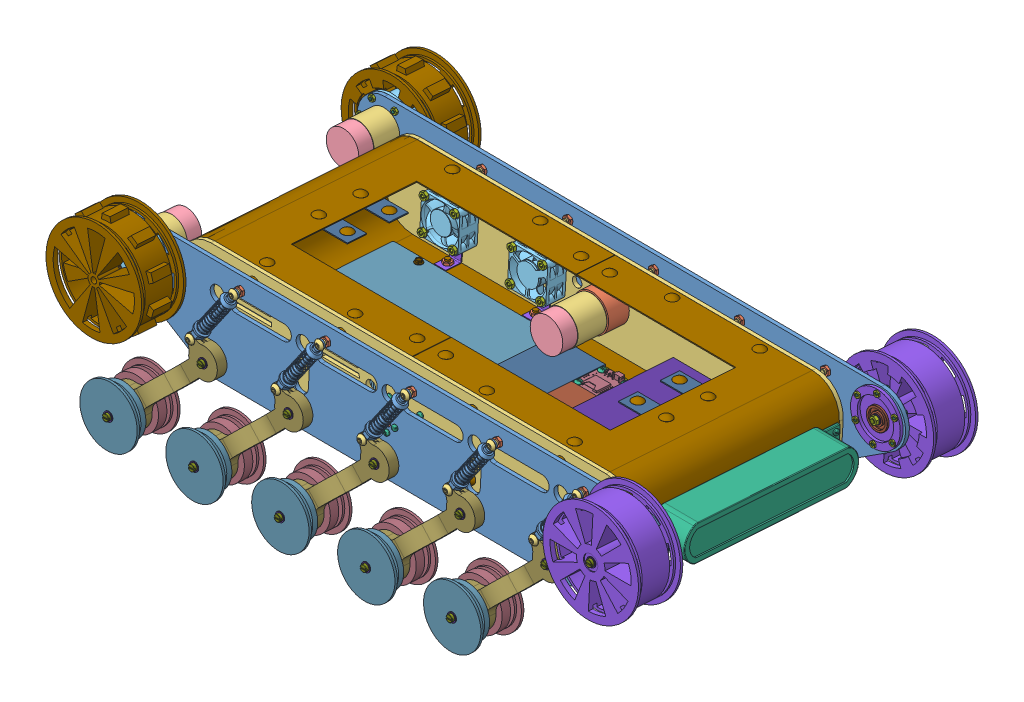
SolidWorks assembly Ensamble_Detallado_2, configuration Predeterminado. Lengths in mm. (continued)
Components (placement in the parent): (continued)
- hex nut jam_am-69: hex nut jam_am [B18.2.4.5M - Hex jam nut,  M5 x 0.8 --D-N] at (182.3196 36.3655 -544.0322) x (0.998179 0.060274 0.002247) z (-0.005872 0.060029 0.998179) size (8 9.24 2.7)
- hex nut jam_am-70: hex nut jam_am [B18.2.4.5M - Hex jam nut,  M5 x 0.8 --D-N] at (92.3211 36.384 -544.5628) x (0.998179 0.060274 0.002247) z (-0.005872 0.060029 0.998179) size (8 9.24 2.7)
- hex nut jam_am-71: hex nut jam_am [B18.2.4.5M - Hex jam nut,  M5 x 0.8 --D-N] at (2.3227 36.4024 -545.0933) x (0.998179 0.060274 0.002247) z (-0.005872 0.060029 0.998179) size (8 9.24 2.7)
- hex nut jam_am-72: hex nut jam_am [B18.2.4.5M - Hex jam nut,  M5 x 0.8 --D-N] at (-87.6757 36.4208 -545.6238) x (0.998179 0.060274 0.002247) z (-0.005872 0.060029 0.998179) size (8 9.24 2.7)
- hex nut jam_am-73: hex nut jam_am [B18.2.4.5M - Hex jam nut,  M5 x 0.8 --D-N] at (182.2802 36.7677 -537.3444) x (0.998179 0.060274 0.002247) z (-0.005872 0.060029 0.998179) size (8 9.24 2.7)
- hex nut jam_am-74: hex nut jam_am [B18.2.4.5M - Hex jam nut,  M5 x 0.8 --D-N] at (92.2818 36.7862 -537.875) x (0.998179 0.060274 0.002247) z (-0.005872 0.060029 0.998179) size (8 9.24 2.7)
- hex nut jam_am-75: hex nut jam_am [B18.2.4.5M - Hex jam nut,  M5 x 0.8 --D-N] at (2.2834 36.8046 -538.4055) x (0.998179 0.060274 0.002247) z (-0.005872 0.060029 0.998179) size (8 9.24 2.7)
- hex nut jam_am-76: hex nut jam_am [B18.2.4.5M - Hex jam nut,  M5 x 0.8 --D-N] at (-87.7151 36.823 -538.936) x (0.998179 0.060274 0.002247) z (-0.005872 0.060029 0.998179) size (8 9.24 2.7)
- Pasador-4: Pasador [Predeterminado] at (98.9679 -93.8939 -530.1771) x (0.998179 0.060274 0.002247) z (-0.005872 0.060029 0.998179) size (8 8 44.5)
- Pasador-5: Pasador [Predeterminado] at (8.9695 -93.8755 -530.7076) x (0.998179 0.060274 0.002247) z (-0.005872 0.060029 0.998179) size (8 8 44.5)
- Pasador-6: Pasador [Predeterminado] at (-81.0289 -93.8571 -531.2382) x (0.998179 0.060274 0.002247) z (-0.005872 0.060029 0.998179) size (8 8 44.5)
- Pasador-7: Pasador [Predeterminado] at (-171.0274 -93.8386 -531.7687) x (0.998179 0.060274 0.002247) z (-0.005872 0.060029 0.998179) size (8 8 44.5)
- Tubo_Pata-2: Tubo_Pata [Predeterminado] at (158.4464 -33.6132 -539.9643) x (0.999983 0.000176 0.005872) z (-0.005872 0.060029 0.998179) size (8 8 11)
- Tubo_Pata-3: Tubo_Pata [Predeterminado] at (68.448 -33.5947 -540.4948) x (0.999983 0.000176 0.005872) z (-0.005872 0.060029 0.998179) size (8 8 11)
- Tubo_Pata-4: Tubo_Pata [Predeterminado] at (-21.5505 -33.5763 -541.0253) x (0.999983 0.000176 0.005872) z (-0.005872 0.060029 0.998179) size (8 8 11)
- Tubo_Pata-5: Tubo_Pata [Predeterminado] at (-111.5489 -33.5579 -541.5558) x (0.999983 0.000176 0.005872) z (-0.005872 0.060029 0.998179) size (8 8 11)
- plain washer - normal_as-30: plain washer - normal_as [AS 1237.1 N - 4] at (100.4952 -109.5074 -789.8036) x (-0.99997 -0.005414 -0.005557) z (0.005872 -0.060029 -0.998179) size (9 9 0.8)
- plain washer - normal_as-31: plain washer - normal_as [AS 1237.1 N - 4] at (10.4967 -109.489 -790.3341) x (-0.99997 -0.005414 -0.005557) z (0.005872 -0.060029 -0.998179) size (9 9 0.8)
- plain washer - normal_as-32: plain washer - normal_as [AS 1237.1 N - 4] at (-79.5017 -109.4705 -790.8646) x (-0.99997 -0.005414 -0.005557) z (0.005872 -0.060029 -0.998179) size (9 9 0.8)
- plain washer - normal_as-33: plain washer - normal_as [AS 1237.1 N - 4] at (-169.5001 -109.4521 -791.3951) x (-0.99997 -0.005414 -0.005557) z (0.005872 -0.060029 -0.998179) size (9 9 0.8)
- Rueda_Resorte2V1.3-20: Rueda_Resorte2V1.3 [Predeterminado] at (100.6067 -110.648 -808.769) x (0.047484 -0.997054 0.06024) z (-0.005872 0.060029 0.998179) size (60 60 20.5)
- Rueda_Resorte2V1.3-21: Rueda_Resorte2V1.3 [Predeterminado] at (10.6083 -110.6295 -809.2995) x (0.047484 -0.997054 0.06024) z (-0.005872 0.060029 0.998179) size (60 60 20.5)
- Rueda_Resorte2V1.3-22: Rueda_Resorte2V1.3 [Predeterminado] at (-79.3901 -110.6111 -809.83) x (0.047484 -0.997054 0.06024) z (-0.005872 0.060029 0.998179) size (60 60 20.5)
- Rueda_Resorte2V1.3-23: Rueda_Resorte2V1.3 [Predeterminado] at (-169.3886 -110.5927 -810.3605) x (0.047484 -0.997054 0.06024) z (-0.005872 0.060029 0.998179) size (60 60 20.5)
- hex nut style 1_am-111: hex nut style 1_am [B18.2.4.1M - Hex nut, Style 1,  M4 x 0.7 --D-N] at (100.4905 -109.4594 -789.005) x (-0.99997 -0.005414 -0.005557) z (0.005872 -0.060029 -0.998179) size (7 8.08 3.2)
- hex nut style 1_am-112: hex nut style 1_am [B18.2.4.1M - Hex nut, Style 1,  M4 x 0.7 --D-N] at (10.492 -109.441 -789.5356) x (-0.99997 -0.005414 -0.005557) z (0.005872 -0.060029 -0.998179) size (7 8.08 3.2)
- hex nut style 1_am-113: hex nut style 1_am [B18.2.4.1M - Hex nut, Style 1,  M4 x 0.7 --D-N] at (-79.5064 -109.4225 -790.0661) x (-0.99997 -0.005414 -0.005557) z (0.005872 -0.060029 -0.998179) size (7 8.08 3.2)
- hex nut style 1_am-114: hex nut style 1_am [B18.2.4.1M - Hex nut, Style 1,  M4 x 0.7 --D-N] at (-169.5048 -109.4041 -790.5966) x (-0.99997 -0.005414 -0.005557) z (0.005872 -0.060029 -0.998179) size (7 8.08 3.2)
- plain washer - normal_as-34: plain washer - normal_as [AS 1237.1 N - 4] at (100.7611 -112.2267 -835.0211) x (-0.99997 -0.005414 -0.005557) z (0.005872 -0.060029 -0.998179) size (9 9 0.8)
- plain washer - normal_as-35: plain washer - normal_as [AS 1237.1 N - 4] at (10.7627 -112.2083 -835.5516) x (-0.99997 -0.005414 -0.005557) z (0.005872 -0.060029 -0.998179) size (9 9 0.8)
- plain washer - normal_as-36: plain washer - normal_as [AS 1237.1 N - 4] at (-79.2357 -112.1898 -836.0821) x (-0.99997 -0.005414 -0.005557) z (0.005872 -0.060029 -0.998179) size (9 9 0.8)
- plain washer - normal_as-37: plain washer - normal_as [AS 1237.1 N - 4] at (-169.2342 -112.1714 -836.6127) x (-0.99997 -0.005414 -0.005557) z (0.005872 -0.060029 -0.998179) size (9 9 0.8)
- cheese head screw_as-16: cheese head screw_as [AS-NZS 1427 CH - M4 x 50-N] at (100.7764 -112.3828 -837.6164) x (-0.005872 0.060029 0.998179) z (-0.99997 -0.005414 -0.005557) size (52.62 7 7)
- cheese head screw_as-17: cheese head screw_as [AS-NZS 1427 CH - M4 x 50-N] at (10.778 -112.3644 -838.1469) x (-0.005872 0.060029 0.998179) z (-0.99997 -0.005414 -0.005557) size (52.62 7 7)
- cheese head screw_as-18: cheese head screw_as [AS-NZS 1427 CH - M4 x 50-N] at (-79.2205 -112.3459 -838.6774) x (-0.005872 0.060029 0.998179) z (-0.99997 -0.005414 -0.005557) size (52.62 7 7)
- cheese head screw_as-19: cheese head screw_as [AS-NZS 1427 CH - M4 x 50-N] at (-169.2189 -112.3275 -839.2079) x (-0.005872 0.060029 0.998179) z (-0.99997 -0.005414 -0.005557) size (52.62 7 7)
- Rueda_ResorteV1.3-24: Rueda_ResorteV1.3 [Predeterminado] at (100.6654 -111.2482 -818.7508) x (0.99997 -0.004709 0.006165) z (0.005872 -0.060029 -0.998179) size (60 60 17)
- Rueda_ResorteV1.3-25: Rueda_ResorteV1.3 [Predeterminado] at (10.667 -111.2298 -819.2813) x (0.99997 -0.004709 0.006165) z (0.005872 -0.060029 -0.998179) size (60 60 17)
- Rueda_ResorteV1.3-26: Rueda_ResorteV1.3 [Predeterminado] at (-79.3314 -111.2114 -819.8118) x (0.99997 -0.004709 0.006165) z (0.005872 -0.060029 -0.998179) size (60 60 17)
- Rueda_ResorteV1.3-27: Rueda_ResorteV1.3 [Predeterminado] at (-169.3299 -111.1929 -820.3423) x (0.99997 -0.004709 0.006165) z (0.005872 -0.060029 -0.998179) size (60 60 17)
- plain washer - normal_as-38: plain washer - normal_as [AS 1237.1 N - 4] at (159.8973 -48.4463 -786.6144) x (-0.998179 -0.060274 -0.002247) z (0.005872 -0.060029 -0.998179) size (9 9 0.8)
- plain washer - normal_as-39: plain washer - normal_as [AS 1237.1 N - 4] at (69.8989 -48.4278 -787.1449) x (-0.998179 -0.060274 -0.002247) z (0.005872 -0.060029 -0.998179) size (9 9 0.8)
- plain washer - normal_as-40: plain washer - normal_as [AS 1237.1 N - 4] at (-20.0996 -48.4094 -787.6754) x (-0.998179 -0.060274 -0.002247) z (0.005872 -0.060029 -0.998179) size (9 9 0.8)
- plain washer - normal_as-41: plain washer - normal_as [AS 1237.1 N - 4] at (-110.098 -48.391 -788.206) x (-0.998179 -0.060274 -0.002247) z (0.005872 -0.060029 -0.998179) size (9 9 0.8)
- hex nut style 1_am-115: hex nut style 1_am [B18.2.4.1M - Hex nut, Style 1,  M4 x 0.7 --D-N] at (159.8926 -48.3982 -785.8159) x (-0.99853 -0.054135 -0.002618) z (0.005872 -0.060029 -0.998179) size (7 8.08 3.2)
- hex nut style 1_am-116: hex nut style 1_am [B18.2.4.1M - Hex nut, Style 1,  M4 x 0.7 --D-N] at (69.8942 -48.3798 -786.3464) x (-0.99853 -0.054135 -0.002618) z (0.005872 -0.060029 -0.998179) size (7 8.08 3.2)
- hex nut style 1_am-117: hex nut style 1_am [B18.2.4.1M - Hex nut, Style 1,  M4 x 0.7 --D-N] at (-20.1043 -48.3614 -786.8769) x (-0.99853 -0.054135 -0.002618) z (0.005872 -0.060029 -0.998179) size (7 8.08 3.2)
- hex nut style 1_am-118: hex nut style 1_am [B18.2.4.1M - Hex nut, Style 1,  M4 x 0.7 --D-N] at (-110.1027 -48.3429 -787.4074) x (-0.99853 -0.054135 -0.002618) z (0.005872 -0.060029 -0.998179) size (7 8.08 3.2)
- plain washer - normal_as-42: plain washer - normal_as [AS 1237.1 N - 4] at (159.993 -49.4247 -802.8847) x (0.958426 -0.284435 0.022743) z (0.005872 -0.060029 -0.998179) size (9 9 0.8)
- plain washer - normal_as-43: plain washer - normal_as [AS 1237.1 N - 4] at (69.9946 -49.4063 -803.4152) x (0.958426 -0.284435 0.022743) z (0.005872 -0.060029 -0.998179) size (9 9 0.8)
- plain washer - normal_as-44: plain washer - normal_as [AS 1237.1 N - 4] at (-20.0039 -49.3879 -803.9458) x (0.958426 -0.284435 0.022743) z (0.005872 -0.060029 -0.998179) size (9 9 0.8)
- plain washer - normal_as-45: plain washer - normal_as [AS 1237.1 N - 4] at (-110.0023 -49.3694 -804.4763) x (0.958426 -0.284435 0.022743) z (0.005872 -0.060029 -0.998179) size (9 9 0.8)
- socket button head cap screw_am-16: socket button head cap screw_am [B18.3.4M - 5 x 0.8 x 10 SBHCS --N] at (145.7758 -35.5561 -805.756) x (-0.005872 0.060029 0.998179) z (-0.100585 -0.993169 0.059136) size (12.75 9.5 9.5)
- socket button head cap screw_am-17: socket button head cap screw_am [B18.3.4M - 5 x 0.8 x 10 SBHCS --N] at (55.7774 -35.5376 -806.2865) x (-0.005872 0.060029 0.998179) z (-0.100585 -0.993169 0.059136) size (12.75 9.5 9.5)
- socket button head cap screw_am-18: socket button head cap screw_am [B18.3.4M - 5 x 0.8 x 10 SBHCS --N] at (-34.2211 -35.5192 -806.817) x (-0.005872 0.060029 0.998179) z (-0.100585 -0.993169 0.059136) size (12.75 9.5 9.5)
- socket button head cap screw_am-19: socket button head cap screw_am [B18.3.4M - 5 x 0.8 x 10 SBHCS --N] at (-124.2195 -35.5008 -807.3475) x (-0.005872 0.060029 0.998179) z (-0.100585 -0.993169 0.059136) size (12.75 9.5 9.5)
- cheese head screw_as-20: cheese head screw_as [AS-NZS 1427 CH - M4 x 20-N] at (160.0083 -49.5808 -805.48) x (-0.005872 0.060029 0.998179) z (0.11687 0.991397 -0.058933) size (22.6 7 7)
- cheese head screw_as-21: cheese head screw_as [AS-NZS 1427 CH - M4 x 20-N] at (70.0098 -49.5624 -806.0105) x (-0.005872 0.060029 0.998179) z (0.11687 0.991397 -0.058933) size (22.6 7 7)
- cheese head screw_as-22: cheese head screw_as [AS-NZS 1427 CH - M4 x 20-N] at (-19.9886 -49.5439 -806.541) x (-0.005872 0.060029 0.998179) z (0.11687 0.991397 -0.058933) size (22.6 7 7)
- cheese head screw_as-23: cheese head screw_as [AS-NZS 1427 CH - M4 x 20-N] at (-109.987 -49.5255 -807.0715) x (-0.005872 0.060029 0.998179) z (0.11687 0.991397 -0.058933) size (22.6 7 7)
- Pieza_Resorte_2V1.5-2: Pieza_Resorte_2V1.5 [Predeterminado] at (100.6361 -110.9481 -813.7599) x (0.005872 -0.060029 -0.998179) z (-0.699298 -0.713776 0.038812) size (30 44.97 120)
- Pieza_Resorte_2V1.5-3: Pieza_Resorte_2V1.5 [Predeterminado] at (10.6376 -110.9297 -814.2904) x (0.005872 -0.060029 -0.998179) z (-0.699298 -0.713776 0.038812) size (30 44.97 120)
- Pieza_Resorte_2V1.5-4: Pieza_Resorte_2V1.5 [Predeterminado] at (-79.3608 -110.9112 -814.8209) x (0.005872 -0.060029 -0.998179) z (-0.699298 -0.713776 0.038812) size (30 44.97 120)
- Pieza_Resorte_2V1.5-5: Pieza_Resorte_2V1.5 [Predeterminado] at (-169.3592 -110.8928 -815.3514) x (0.005872 -0.060029 -0.998179) z (-0.699298 -0.713776 0.038812) size (30 44.97 120)
- hex nut jam_am-77: hex nut jam_am [B18.2.4.5M - Hex jam nut,  M5 x 0.8 --D-N] at (183.7546 21.6945 -787.9873) x (0.998179 0.060274 0.002247) z (-0.005872 0.060029 0.998179) size (8 9.24 2.7)
- hex nut jam_am-78: hex nut jam_am [B18.2.4.5M - Hex jam nut,  M5 x 0.8 --D-N] at (93.7562 21.7129 -788.5178) x (0.998179 0.060274 0.002247) z (-0.005872 0.060029 0.998179) size (8 9.24 2.7)
- hex nut jam_am-79: hex nut jam_am [B18.2.4.5M - Hex jam nut,  M5 x 0.8 --D-N] at (3.7577 21.7314 -789.0483) x (0.998179 0.060274 0.002247) z (-0.005872 0.060029 0.998179) size (8 9.24 2.7)
- hex nut jam_am-80: hex nut jam_am [B18.2.4.5M - Hex jam nut,  M5 x 0.8 --D-N] at (-86.2407 21.7498 -789.5788) x (0.998179 0.060274 0.002247) z (-0.005872 0.060029 0.998179) size (8 9.24 2.7)
- Resorte-7: Resorte [Predeterminado] at (153.036 -24.3547 -798.6227) x (-0.827134 0.560678 -0.038584) z (-0.561974 -0.825855 0.04636) size (14 14 75.95)
- Resorte-8: Resorte [Predeterminado] at (63.0375 -24.3363 -799.1533) x (-0.827134 0.560678 -0.038584) z (-0.561974 -0.825855 0.04636) size (14 14 75.95)
- Resorte-9: Resorte [Predeterminado] at (-26.9609 -24.3179 -799.6838) x (-0.827134 0.560678 -0.038584) z (-0.561974 -0.825855 0.04636) size (14 14 75.95)
- Resorte-10: Resorte [Predeterminado] at (-116.9593 -24.2994 -800.2143) x (-0.827134 0.560678 -0.038584) z (-0.561974 -0.825855 0.04636) size (14 14 75.95)
- hex nut jam_am-81: hex nut jam_am [B18.2.4.5M - Hex jam nut,  M5 x 0.8 --D-N] at (183.7939 21.2923 -794.6751) x (0.998179 0.060274 0.002247) z (-0.005872 0.060029 0.998179) size (8 9.24 2.7)
- hex nut jam_am-82: hex nut jam_am [B18.2.4.5M - Hex jam nut,  M5 x 0.8 --D-N] at (93.7955 21.3107 -795.2056) x (0.998179 0.060274 0.002247) z (-0.005872 0.060029 0.998179) size (8 9.24 2.7)
- hex nut jam_am-83: hex nut jam_am [B18.2.4.5M - Hex jam nut,  M5 x 0.8 --D-N] at (3.7971 21.3292 -795.7361) x (0.998179 0.060274 0.002247) z (-0.005872 0.060029 0.998179) size (8 9.24 2.7)
- hex nut jam_am-84: hex nut jam_am [B18.2.4.5M - Hex jam nut,  M5 x 0.8 --D-N] at (-86.2014 21.3476 -796.2666) x (0.998179 0.060274 0.002247) z (-0.005872 0.060029 0.998179) size (8 9.24 2.7)
- socket button head cap screw_am-20: socket button head cap screw_am [B18.3.4M - 5 x 0.8 x 16 SBHCS --N] at (183.8541 20.677 -804.9064) x (-0.005872 0.060029 0.998179) z (0.095597 0.993658 -0.059195) size (18.75 9.5 9.5)
- socket button head cap screw_am-21: socket button head cap screw_am [B18.3.4M - 5 x 0.8 x 16 SBHCS --N] at (93.8557 20.6955 -805.4369) x (-0.005872 0.060029 0.998179) z (0.095597 0.993658 -0.059195) size (18.75 9.5 9.5)
- socket button head cap screw_am-22: socket button head cap screw_am [B18.3.4M - 5 x 0.8 x 16 SBHCS --N] at (3.8573 20.7139 -805.9675) x (-0.005872 0.060029 0.998179) z (0.095597 0.993658 -0.059195) size (18.75 9.5 9.5)
- socket button head cap screw_am-23: socket button head cap screw_am [B18.3.4M - 5 x 0.8 x 16 SBHCS --N] at (-86.1412 20.7323 -806.498) x (-0.005872 0.060029 0.998179) z (0.095597 0.993658 -0.059195) size (18.75 9.5 9.5)
- Tubo_Pata-6: Tubo_Pata [Predeterminado] at (249.9603 -49.125 -797.0639) x (0.997189 0.074911 0.001361) z (-0.005872 0.060029 0.998179) size (8 8 11)
- Pasador-8: Pasador [Predeterminado] at (100.7565 -112.1787 -834.2226) x (0.999795 0.019701 0.004696) z (-0.005872 0.060029 0.998179) size (8 8 44.5)
- Pasador-9: Pasador [Predeterminado] at (10.758 -112.1603 -834.7531) x (0.999795 0.019701 0.004696) z (-0.005872 0.060029 0.998179) size (8 8 44.5)
- Pasador-10: Pasador [Predeterminado] at (-79.2404 -112.1418 -835.2836) x (0.999795 0.019701 0.004696) z (-0.005872 0.060029 0.998179) size (8 8 44.5)
- Pasador-11: Pasador [Predeterminado] at (-169.2389 -112.1234 -835.8141) x (0.999795 0.019701 0.004696) z (-0.005872 0.060029 0.998179) size (8 8 44.5)
- Tubo_Pata-7: Tubo_Pata [Predeterminado] at (159.9619 -49.1066 -797.5944) x (0.997189 0.074911 0.001361) z (-0.005872 0.060029 0.998179) size (8 8 11)
- Tubo_Pata-8: Tubo_Pata [Predeterminado] at (69.9635 -49.0881 -798.1249) x (0.997189 0.074911 0.001361) z (-0.005872 0.060029 0.998179) size (8 8 11)
- Tubo_Pata-9: Tubo_Pata [Predeterminado] at (-20.035 -49.0697 -798.6554) x (0.997189 0.074911 0.001361) z (-0.005872 0.060029 0.998179) size (8 8 11)
- Tubo_Pata-10: Tubo_Pata [Predeterminado] at (-110.0334 -49.0513 -799.1859) x (0.997189 0.074911 0.001361) z (-0.005872 0.060029 0.998179) size (8 8 11)
Mates (geometry in assembly coordinates):
- Concéntrica49: concentric aligned: cylinder of Perfil_IzquierdoV2.2-1 through (-191.5397 22.5977 -541.3962) axis (0.005872 -0.060029 -0.998179) radius 17.4; cylinder of Motor_4-1/Motor_2-1 through (-191.5397 22.5977 -541.3962) axis (0.005872 -0.060029 -0.998179) radius 17.4
- Concéntrica65: concentric anti-aligned: cylinder of Motor_4-1/Motor_1-1 through (-191.666 23.8883 -519.9353) axis (0.005872 -0.060029 -0.998179) radius 18.4; cylinder of Tapa_motor-1 through (-191.5397 22.5977 -541.3962) axis (-0.005872 0.060029 0.998179) radius 18.4
- Concéntrica66: concentric anti-aligned: cylinder of Motor_4-1/Motor_1-1 through (-191.7051 17.2611 -513.526) axis (0.005872 -0.060029 -0.998179) radius 6; cylinder of Tapa_motor-1 through (-191.6699 16.9009 -519.5151) axis (-0.005872 0.060029 0.998179) radius 6
- Coincidente27: coincident anti-aligned: plane of Motor_4-1/Motor_1-1 through (-191.666 23.8883 -519.9353) normal (-0.005872 0.060029 0.998179); plane of Tapa_motor-1 through (-191.666 23.8883 -519.9353) normal (0.005872 -0.060029 -0.998179)
- Concéntrica67: concentric aligned: cylinder of Tapa_motor-1 through (-183.9086 37.2859 -520.6954) axis (-0.005872 0.060029 0.998179) radius 1.5; cylinder of pan head tapping screw_am-8 through (-183.9391 37.598 -515.5049) axis (-0.005872 0.060029 0.998179) radius 1.5
- Coincidente28: coincident anti-aligned: plane of Tapa_motor-1 through (-191.6836 24.0684 -516.9408) normal (-0.005872 0.060029 0.998179); plane of pan head tapping screw_am-8 through (-181.1518 37.09 -517.6619) normal (0.005872 -0.060029 -0.998179)
- Coincidente29: coincident anti-aligned: plane of Perfil_IzquierdoV2.2-1 through (258.432 -33.3713 -535.3834) normal (-0.005872 0.060029 0.998179); plane of Motor_4-1/Motor_1-1 through (-191.5397 22.5977 -541.3962) normal (0.005872 -0.060029 -0.998179)
- Concéntrica68: concentric anti-aligned: cylinder of Tapa_motor-1 through (-215.2969 22.7643 -538.5405) axis (0.005872 -0.060029 -0.998179) radius 1.5; cylinder of pan head tapping screw_am-14 through (-215.3099 22.8964 -536.3445) axis (-0.005872 0.060029 0.998179) radius 1.5
- Coincidente30: coincident anti-aligned: plane of Tapa_motor-1 through (-191.5573 22.7777 -538.4016) normal (-0.005872 0.060029 0.998179); plane of pan head tapping screw_am-14 through (-216.9417 25.0256 -538.6861) normal (0.005872 -0.060029 -0.998179)
- Coincidente32: coincident anti-aligned: plane of Perfil_IzquierdoV2.2-1 through (258.4555 -33.6114 -539.3761) normal (0.005872 -0.060029 -0.998179); plane of hex nut style 1_am-1 through (-220.5915 23.6737 -545.6391) normal (-0.005872 0.060029 0.998179)
- Coincidente40: coincident anti-aligned: plane of Perfil_IzquierdoV2.2-1 through (258.4555 -33.6114 -539.3761) normal (0.005872 -0.060029 -0.998179); plane of Pieza_Fijacion-1 through (328.1255 22.8785 -542.3635) normal (-0.005872 0.060029 0.998179)
- Concéntrica102: concentric anti-aligned: cylinder of Perfil_IzquierdoV2.2-1 through (348.0015 33.1166 -548.8732) axis (-0.005872 0.060029 0.998179) radius 1.5; cylinder of Pieza_Fijacion-1 through (347.9721 33.4167 -543.8823) axis (0.005872 -0.060029 -0.998179) radius 1.5
- Concéntrica103: concentric anti-aligned: cylinder of Pieza_Fijacion-1 through (328.863 45.2663 -544.7073) axis (0.005872 -0.060029 -0.998179) radius 1.5; cylinder of pan head tapping screw_am-20 through (328.8149 45.7585 -536.5222) axis (-0.005872 0.060029 0.998179) radius 1.5
- Concéntrica104: concentric aligned: cylinder of pan head tapping screw_am-20 through (328.8149 45.7585 -536.5222) axis (-0.005872 0.060029 0.998179) radius 1.5; cylinder of hex nut style 1_am-7 through (328.8888 45.0022 -549.0993) axis (-0.005872 0.060029 0.998179) radius 1.25
- Coincidente49: coincident anti-aligned: plane of Pieza_Fijacion-1 through (328.1431 22.6984 -545.358) normal (0.005872 -0.060029 -0.998179); plane of hex nut style 1_am-7 through (331.2837 50.0825 -546.9864) normal (-0.005872 0.060029 0.998179)
- Concéntrica11732: concentric aligned: circle of Ensamble_internoV1.1-1/ChasisV1.7-1; circle of Soporte_zed-1
- Concéntrica11734: concentric aligned: circle of Ensamble_internoV1.1-1/ChasisV1.7-1; circle of Soporte_zed-1
- Coincidente860: coincident anti-aligned: plane of fan-2 through (-107.8082 -13.9539 -581.3331) normal (0.005872 -0.060029 -0.998179); plane of hex nut style 1 gradeab_bsi-1 through (-107.4111 22.0038 -583.4932) normal (-0.005872 0.060029 0.998179)
- Coincidente865: coincident anti-aligned: plane of fan-2 through (-107.8082 -13.9539 -581.3331) normal (0.005872 -0.060029 -0.998179); plane of hex nut style 1 gradeab_bsi-2 through (-111.0961 -11.6092 -581.4934) normal (-0.005872 0.060029 0.998179)
- Coincidente867: coincident anti-aligned: plane of fan-2 through (-107.8082 -13.9539 -581.3331) normal (0.005872 -0.060029 -0.998179); plane of hex nut style 1 gradeab_bsi-3 through (-75.0913 -9.9779 -581.3797) normal (-0.005872 0.060029 0.998179)
- Coincidente869: coincident anti-aligned: plane of fan-2 through (-107.8082 -13.9539 -581.3331) normal (0.005872 -0.060029 -0.998179); plane of hex nut style 1 gradeab_bsi-4 through (-72.5268 20.3571 -583.1889) normal (-0.005872 0.060029 0.998179)
- Coincidente880: coincident anti-aligned: plane of fan-1 through (16.1896 -13.967 -580.6029) normal (0.005872 -0.060029 -0.998179); plane of hex nut style 1 gradeab_bsi-5 through (-12.5278 20.3326 -582.8345) normal (-0.005872 0.060029 0.998179)
- Coincidente882: coincident anti-aligned: plane of fan-1 through (16.1896 -13.967 -580.6029) normal (0.005872 -0.060029 -0.998179); plane of hex nut style 1 gradeab_bsi-7 through (16.9128 21.9456 -582.7584) normal (-0.005872 0.060029 0.998179)
- Coincidente884: coincident anti-aligned: plane of fan-1 through (16.1896 -13.967 -580.6029) normal (0.005872 -0.060029 -0.998179); plane of hex nut style 1 gradeab_bsi-6 through (-12.6058 -16.4304 -580.6241) normal (-0.005872 0.060029 0.998179)
- Coincidente886: coincident anti-aligned: plane of fan-1 through (16.1896 -13.967 -580.6029) normal (0.005872 -0.060029 -0.998179); plane of hex nut style 1 gradeab_bsi-8 through (19.3936 -16.4247 -580.4362) normal (-0.005872 0.060029 0.998179)
- Paralelo21: parallel anti-aligned: plane of Ensamble_internoV1.1-1/ChasisV1.7-1 through (-137.1797 30.8436 -774.5465) normal (0.000029 -0.998197 0.06003); plane of Pieza_union_chasis-1 through (-98.4876 43.5668 -565.7028) normal (-0.000029 0.998197 -0.06003)
- Concéntrica117781: concentric aligned: cylinder of Ensamble_internoV1.1-1/ChasisV1.7-1 through (-92.3683 -39.9233 -568.6604) axis (-0.000029 0.998197 -0.06003) radius 2.5; cylinder of round head bolt_ai-8 through (-92.3708 46.562 -573.8615) axis (-0.000029 0.998197 -0.06003) radius 5.7658
- Coincidente892: coincident aligned: plane of Ensamble_internoV1.1-1/ChasisV1.7-1 through (-137.1798 31.8418 -774.6065) normal (-0.000029 0.998197 -0.06003); circle of round head bolt_ai-8
- Concéntrica117831: concentric aligned: cylinder of round head bolt_ai-8 through (-92.3708 46.562 -573.8615) axis (-0.000029 0.998197 -0.06003) radius 2.413; cylinder of hex nut jam_am-6 through (-92.37 17.0984 -572.0896) axis (-0.000029 0.998197 -0.06003) radius 2.5
- Coincidente893: coincident anti-aligned: plane of Pieza_union_chasis-1 through (-86.3938 41.6127 -581.5433) normal (0.000029 -0.998197 0.06003); plane of hex nut jam_am-6 through (-92.0581 41.8141 -578.1925) normal (-0.000029 0.998197 -0.06003)
- Concéntrica11785: concentric anti-aligned: cylinder of round head bolt_ai-9 through (-92.5322 32.0495 -557.3196) axis (-0.005872 0.060029 0.998179) radius 2.413; cylinder of hex nut jam_am-7 through (-92.4873 31.5908 -564.9473) axis (0.005872 -0.060029 -0.998179) radius 2.1
- Coincidente895: coincident anti-aligned: plane of Pieza_union_chasis-1 through (-92.4877 43.5691 -565.6676) normal (0.005872 -0.060029 -0.998179); plane of hex nut jam_am-7 through (-92.1747 26.991 -564.6688) normal (-0.005872 0.060029 0.998179)
- Paralelo24: parallel anti-aligned: line of Ensamble_internoV1.1-1/ChasisV1.7-1 through (-137.1798 31.8418 -774.6065) axis (0.999983 0.000382 0.005859); line of Puerta-1 through (235.8156 42.1896 -602.7246) axis (-0.999983 -0.000382 -0.005859)
- Coincidente911: coincident anti-aligned: plane of Ensamble_internoV1.1-1/ChasisV1.7-1 through (235.8158 34.204 -602.2444) normal (-0.999983 -0.000382 -0.005859); plane of Puerta-1 through (236.1973 38.2877 -667.6063) normal (0.999983 0.000382 0.005859)
- Coincidente912: coincident anti-aligned: plane of Ensamble_internoV1.1-1/ChasisV1.7-1 through (236.5792 26.4002 -732.0077) normal (-0.005872 0.060029 0.998179); plane of Puerta-1 through (69.5818 34.322 -733.4664) normal (0.005872 -0.060029 -0.998179)
- Coincidente913: coincident aligned: plane of Ensamble_internoV1.1-1/ChasisV1.7-1 through (-137.1798 31.8418 -774.6065) normal (-0.000029 0.998197 -0.06003); plane of Puerta-1 through (69.2001 38.2239 -668.5848) normal (-0.000029 0.998197 -0.06003)
- Coincidente915: coincident anti-aligned: plane of Ensamble_internoV1.1-1/ChasisV1.7-1 through (-137.1797 30.8436 -774.5465) normal (0.000029 -0.998197 0.06003); plane of lamina_union-3 through (68.7011 42.3282 -583.6795) normal (-0.000029 0.998197 -0.06003)
- Paralelo26: parallel anti-aligned: line of Ensamble_internoV1.1-1/ChasisV1.7-1 through (275.58 44.606 -562.5631) axis (-0.999983 -0.000382 -0.005859); line of lamina_union-3 through (43.6428 41.9207 -573.7842) axis (0.999983 0.000382 0.005859)
- Concéntrica11792: concentric aligned: circle of Ensamble_internoV1.1-1/ChasisV1.7-1; circle of lamina_union-3
- Coincidente921: coincident anti-aligned: plane of Ensamble_internoV1.1-1/ChasisV1.7-1 through (-137.1797 30.8436 -774.5465) normal (0.000029 -0.998197 0.06003); plane of lamina_union-2 through (236.0701 38.5901 -645.919) normal (-0.000029 0.998197 -0.06003)
- Paralelo28: parallel anti-aligned: line of Ensamble_internoV1.1-1/ChasisV1.7-1 through (70.3167 30.9229 -773.3306) axis (0.999983 0.000382 0.005859); line of lamina_union-2 through (261.011 38.2017 -635.7307) axis (-0.999983 -0.000382 -0.005859)
- Concéntrica11794: concentric aligned: circle of Ensamble_internoV1.1-1/ChasisV1.7-1; circle of lamina_union-2
- Coincidente925: coincident anti-aligned: plane of Ensamble_internoV1.1-1/ChasisV1.7-1 through (-137.1797 30.8436 -774.5465) normal (0.000029 -0.998197 0.06003); plane of lamina_union-4 through (-97.9242 38.4626 -647.876) normal (-0.000029 0.998197 -0.06003)
- Paralelo29: parallel anti-aligned: line of Ensamble_internoV1.1-1/ChasisV1.7-1 through (-137.1797 30.8436 -774.5465) axis (0.999983 0.000382 0.005859); line of lamina_union-4 through (-72.9833 38.0742 -637.6877) axis (-0.999983 -0.000382 -0.005859)
- Concéntrica11795: concentric aligned: circle of Ensamble_internoV1.1-1/ChasisV1.7-1; circle of lamina_union-4
- Concéntrica117961: concentric aligned: circle of Ensamble_internoV1.1-1/ChasisV1.7-1; cylinder of round head bolt_ai-28 through (83.7007 45.9689 -583.8102) axis (-0.000029 0.998197 -0.06003) radius 2.413
- Coincidente9281: coincident anti-aligned: plane of Ensamble_internoV1.1-1/ChasisV1.7-1 through (-137.1798 31.8418 -774.6065) normal (-0.000029 0.998197 -0.06003); plane of round head bolt_ai-28 through (89.4666 43.3322 -583.6516) normal (0.000029 -0.998197 0.06003)
- Concéntrica117971: concentric aligned: cylinder of round head bolt_ai-28 through (83.7007 45.9689 -583.8102) axis (-0.000029 0.998197 -0.06003) radius 2.413; cylinder of hex nut jam_am-26 through (83.7009 38.6406 -583.3695) axis (-0.000029 0.998197 -0.06003) radius 2.1
- Coincidente9301: coincident anti-aligned: plane of lamina_union-3 through (68.7011 41.33 -583.6195) normal (0.000029 -0.998197 0.06003); plane of hex nut jam_am-26 through (80.1611 41.1575 -586.4933) normal (-0.000029 0.998197 -0.06003)
- Concéntrica117981: concentric aligned: circle of Ensamble_internoV1.1-1/ChasisV1.7-1; cylinder of round head bolt_ai-31 through (53.7012 45.9575 -583.986) axis (-0.000029 0.998197 -0.06003) radius 2.413
- Coincidente9311: coincident anti-aligned: plane of Ensamble_internoV1.1-1/ChasisV1.7-1 through (-137.1798 31.8418 -774.6065) normal (-0.000029 0.998197 -0.06003); plane of round head bolt_ai-31 through (59.4671 43.3208 -583.8274) normal (0.000029 -0.998197 0.06003)
- Concéntrica117991: concentric aligned: cylinder of round head bolt_ai-31 through (53.7012 45.9575 -583.986) axis (-0.000029 0.998197 -0.06003) radius 2.413; cylinder of hex nut jam_am-27 through (53.7014 38.6291 -583.5453) axis (-0.000029 0.998197 -0.06003) radius 2.1
- Coincidente9321: coincident anti-aligned: plane of lamina_union-3 through (68.7011 41.33 -583.6195) normal (0.000029 -0.998197 0.06003); plane of hex nut jam_am-27 through (54.4193 41.0504 -588.2618) normal (-0.000029 0.998197 -0.06003)
- Concéntrica118011: concentric aligned: circle of Ensamble_internoV1.1-1/ChasisV1.7-1; cylinder of round head bolt_ai-30 through (251.0697 42.2309 -646.0497) axis (-0.000029 0.998197 -0.06003) radius 2.413
- Coincidente9331: coincident anti-aligned: plane of Ensamble_internoV1.1-1/ChasisV1.7-1 through (-137.1798 31.8418 -774.6065) normal (-0.000029 0.998197 -0.06003); plane of round head bolt_ai-30 through (256.8356 39.5942 -645.8912) normal (0.000029 -0.998197 0.06003)
- Coincidente9341: coincident anti-aligned: plane of lamina_union-2 through (236.0701 37.5919 -645.859) normal (0.000029 -0.998197 0.06003); plane of hex nut jam_am-24 through (251.3825 37.321 -650.371) normal (-0.000029 0.998197 -0.06003)
- Concéntrica118031: concentric aligned: cylinder of hex nut jam_am-24 through (251.0699 34.9025 -645.609) axis (-0.000029 0.998197 -0.06003) radius 2.1; cylinder of round head bolt_ai-30 through (251.0697 42.2309 -646.0497) axis (-0.000029 0.998197 -0.06003) radius 2.413
- Concéntrica118051: concentric anti-aligned: circle of lamina_union-2; cylinder of hex nut jam_am-28 through (221.0704 34.8911 -645.7848) axis (-0.000029 0.998197 -0.06003) radius 2.1
- Concéntrica118061: concentric aligned: cylinder of round head bolt_ai-29 through (221.0702 42.2194 -646.2255) axis (-0.000029 0.998197 -0.06003) radius 2.413; cylinder of hex nut jam_am-28 through (221.0704 34.8911 -645.7848) axis (-0.000029 0.998197 -0.06003) radius 2.1
- Coincidente9361: coincident anti-aligned: plane of lamina_union-2 through (236.0701 37.5919 -645.859) normal (0.000029 -0.998197 0.06003); plane of hex nut jam_am-28 through (222.5835 37.3243 -650.3029) normal (-0.000029 0.998197 -0.06003)
- Coincidente9371: coincident anti-aligned: plane of Puerta-1 through (69.2001 38.2239 -668.5848) normal (-0.000029 0.998197 -0.06003); plane of round head bolt_ai-29 through (226.8361 39.5827 -646.0669) normal (0.000029 -0.998197 0.06003)
- Concéntrica118071: concentric aligned: circle of Puerta-1; cylinder of round head bolt_ai-27 through (-82.9245 42.1033 -648.0067) axis (-0.000029 0.998197 -0.06003) radius 2.413
- Coincidente9381: coincident anti-aligned: plane of Puerta-1 through (69.2001 38.2239 -668.5848) normal (-0.000029 0.998197 -0.06003); plane of round head bolt_ai-27 through (-77.1587 39.4667 -647.8482) normal (0.000029 -0.998197 0.06003)
- Concéntrica118081: concentric aligned: cylinder of round head bolt_ai-27 through (-82.9245 42.1033 -648.0067) axis (-0.000029 0.998197 -0.06003) radius 2.413; cylinder of hex nut jam_am-29 through (-82.9243 34.775 -647.566) axis (-0.000029 0.998197 -0.06003) radius 2.1
- Coincidente9401: coincident anti-aligned: plane of lamina_union-4 through (-97.9241 37.4644 -647.816) normal (0.000029 -0.998197 0.06003); plane of hex nut jam_am-29 through (-81.6621 37.2034 -652.1631) normal (-0.000029 0.998197 -0.06003)
- Concéntrica118091: concentric aligned: circle of Ensamble_internoV1.1-1/ChasisV1.7-1; cylinder of round head bolt_ai-26 through (-112.924 42.0919 -648.1825) axis (-0.000029 0.998197 -0.06003) radius 2.413
- Coincidente9411: coincident anti-aligned: plane of Ensamble_internoV1.1-1/ChasisV1.7-1 through (-137.1798 31.8418 -774.6065) normal (-0.000029 0.998197 -0.06003); plane of round head bolt_ai-26 through (-107.1581 39.4552 -648.024) normal (0.000029 -0.998197 0.06003)
- Concéntrica118101: concentric aligned: cylinder of round head bolt_ai-26 through (-112.924 42.0919 -648.1825) axis (-0.000029 0.998197 -0.06003) radius 2.413; cylinder of hex nut jam_am-25 through (-112.9238 34.7635 -647.7418) axis (-0.000029 0.998197 -0.06003) radius 2.1
- Coincidente9421: coincident anti-aligned: plane of lamina_union-4 through (-97.9241 37.4644 -647.816) normal (0.000029 -0.998197 0.06003); plane of hex nut jam_am-25 through (-114.6857 37.2023 -652.1658) normal (-0.000029 0.998197 -0.06003)
- Concéntrica118103: concentric anti-aligned: cylinder of instrument ball bearing_68_am-5 through (188.7043 -91.2328 -485.0904) axis (0.005872 -0.060029 -0.998179) radius 11; cylinder of Pieza_ResorteV1.5-6 through (188.8548 -92.7718 -510.6812) axis (-0.005872 0.060029 0.998179) radius 11
- Concéntrica118104: concentric anti-aligned: cylinder of instrument ball bearing_68_am-5 through (188.7043 -91.2328 -485.0904) axis (0.005872 -0.060029 -0.998179) radius 4; cylinder of Rueda_ResorteV1.3-17 through (188.7168 -91.3612 -487.224) axis (-0.005872 0.060029 0.998179) radius 4
- Coincidente9423: coincident anti-aligned: plane of instrument ball bearing_68_am-5 through (194.2926 -89.6009 -502.3244) normal (-0.005872 0.060029 0.998179); plane of Rueda_ResorteV1.3-17 through (188.8049 -92.2616 -502.1967) normal (0.005872 -0.060029 -0.998179)
- Coincidente9430: coincident anti-aligned: plane of Pieza_ResorteV1.5-6 through (212.189 -79.5957 -501.3181) normal (-0.005872 0.060029 0.998179); plane of Rueda_ResorteV1.3-17 through (188.7961 -92.1715 -500.6994) normal (0.005872 -0.060029 -0.998179)
- Concéntrica118112: concentric aligned: cylinder of instrument ball bearing_68_am-5 through (188.7043 -91.2328 -485.0904) axis (0.005872 -0.060029 -0.998179) radius 4; cylinder of Rueda_Resorte2V1.3-13 through (188.9546 -93.7923 -527.6503) axis (0.005872 -0.060029 -0.998179) radius 4
- Coincidente9432: coincident anti-aligned: plane of instrument ball bearing_68_am-5 through (192.7144 -90.8062 -509.274) normal (0.005872 -0.060029 -0.998179); plane of Rueda_Resorte2V1.3-13 through (188.846 -92.6818 -509.1839) normal (-0.005872 0.060029 0.998179)
- Concéntrica118113: concentric anti-aligned: cylinder of Rueda_ResorteV1.3-17 through (188.7168 -91.3612 -487.224) axis (-0.005872 0.060029 0.998179) radius 4; cylinder of Pasador-1 through (188.7051 -91.2411 -485.2276) axis (0.005872 -0.060029 -0.998179) radius 4
- Concéntrica118123: concentric aligned: cylinder of Pieza_Resorte_2V1.5-1 through (190.6052 -110.6664 -808.2385) axis (0.005872 -0.060029 -0.998179) radius 11; cylinder of instrument ball bearing_68_am-6 through (190.5133 -109.7277 -792.6294) axis (0.005872 -0.060029 -0.998179) radius 11
- Concéntrica118127: concentric aligned: cylinder of cheese head screw_as-3 through (190.7748 -112.4012 -837.0859) axis (0.005872 -0.060029 -0.998179) radius 2; cylinder of Pasador-2 through (190.4936 -109.5258 -789.2731) axis (0.005872 -0.060029 -0.998179) radius 2
- Concéntrica118128: concentric aligned: cylinder of cheese head screw_as-3 through (190.7748 -112.4012 -837.0859) axis (0.005872 -0.060029 -0.998179) radius 2; cylinder of plain washer - normal_as-4 through (190.7596 -112.2451 -834.4906) axis (0.005872 -0.060029 -0.998179) radius 2.15
- Coincidente9444: coincident anti-aligned: plane of cheese head screw_as-3 through (190.7418 -108.7515 -834.7008) normal (-0.005872 0.060029 0.998179); plane of plain washer - normal_as-4 through (188.6096 -112.2568 -834.5025) normal (0.005872 -0.060029 -0.998179)
- Concéntrica118129: concentric aligned: cylinder of cheese head screw_as-3 through (190.7748 -112.4012 -837.0859) axis (0.005872 -0.060029 -0.998179) radius 2; cylinder of plain washer - normal_as-3 through (190.4936 -109.5258 -789.2731) axis (0.005872 -0.060029 -0.998179) radius 2.15
- Concéntrica118130: concentric aligned: cylinder of cheese head screw_as-3 through (190.7748 -112.4012 -837.0859) axis (0.005872 -0.060029 -0.998179) radius 2; cylinder of hex nut style 1_am-63 through (190.4701 -109.2857 -785.2803) axis (0.005872 -0.060029 -0.998179) radius 1.65
- Coincidente9447: coincident anti-aligned: plane of hex nut style 1_am-63 through (190.4684 -105.4437 -788.7172) normal (0.005872 -0.060029 -0.998179); plane of plain washer - normal_as-3 through (188.339 -109.4895 -788.4865) normal (-0.005872 0.060029 0.998179)
- Coincidente9448: coincident aligned: plane of Rueda_Resorte2V1.3-13 through (188.9664 -93.9124 -529.6466) normal (0.005872 -0.060029 -0.998179); plane of Pasador-1 through (188.9664 -93.9124 -529.6466) normal (0.005872 -0.060029 -0.998179)
- Coincidente9449: coincident anti-aligned: plane of Rueda_Resorte2V1.3-13 through (188.9664 -93.9124 -529.6466) normal (0.005872 -0.060029 -0.998179); plane of plain washer - normal_as-1 through (186.8203 -94.042 -529.6514) normal (-0.005872 0.060029 0.998179)
- Concéntrica118138: concentric aligned: cylinder of Pasador-1 through (188.7051 -91.2411 -485.2276) axis (0.005872 -0.060029 -0.998179) radius 2; circle of plain washer - normal_as-1
- Coincidente9450: coincident anti-aligned: plane of Rueda_ResorteV1.3-17 through (188.7051 -91.2411 -485.2276) normal (-0.005872 0.060029 0.998179); plane of plain washer - normal_as-2 through (186.559 -91.3707 -485.2325) normal (0.005872 -0.060029 -0.998179)
- Concéntrica118139: concentric aligned: cylinder of Pasador-1 through (188.7051 -91.2411 -485.2276) axis (0.005872 -0.060029 -0.998179) radius 2; cylinder of plain washer - normal_as-2 through (188.7051 -91.2411 -485.2276) axis (0.005872 -0.060029 -0.998179) radius 2.15
- Concéntrica118140: concentric anti-aligned: cylinder of Pasador-1 through (188.7051 -91.2411 -485.2276) axis (0.005872 -0.060029 -0.998179) radius 2; cylinder of cheese head screw_as-2 through (188.6851 -91.037 -481.8338) axis (-0.005872 0.060029 0.998179) radius 2
- Coincidente9451: coincident anti-aligned: plane of cheese head screw_as-2 through (188.9105 -94.6804 -484.2181) normal (0.005872 -0.060029 -0.998179); plane of plain washer - normal_as-2 through (186.5543 -91.3227 -484.4339) normal (-0.005872 0.060029 0.998179)
- Coincidente9452: coincident anti-aligned: plane of plain washer - normal_as-1 through (186.825 -94.09 -530.45) normal (0.005872 -0.060029 -0.998179); plane of hex nut style 1_am-62 through (188.7285 -89.9336 -530.6887) normal (-0.005872 0.060029 0.998179)
- Concéntrica118141: concentric anti-aligned: cylinder of cheese head screw_as-2 through (188.6851 -91.037 -481.8338) axis (-0.005872 0.060029 0.998179) radius 2; cylinder of hex nut style 1_am-62 through (188.9711 -93.9604 -530.4452) axis (0.005872 -0.060029 -0.998179) radius 1.65
- Concéntrica118142: concentric anti-aligned: circle of Pieza_Resorte_2V1.5-1; cylinder of Resorte-2 through (235.7199 -35.0192 -795.9923) axis (0.005872 -0.060029 -0.998179) radius 2.4
- Coincidente9454: coincident anti-aligned: plane of Pieza_Resorte_2V1.5-1 through (234.5833 -42.8783 -798.5318) normal (-0.005872 0.060029 0.998179); plane of Resorte-2 through (235.7375 -35.1993 -798.9868) normal (0.005872 -0.060029 -0.998179)
- Concéntrica118143: concentric anti-aligned: cylinder of Pieza_ResorteV1.5-6 through (234.1839 -19.3157 -534.8686) axis (-0.005872 0.060029 0.998179) radius 2.4; cylinder of Resorte-1 through (234.1457 -18.9255 -528.3804) axis (0.005872 -0.060029 -0.998179) radius 2.4
- Coincidente9455: coincident anti-aligned: plane of Pieza_ResorteV1.5-6 through (233.0091 -26.7846 -530.9199) normal (-0.005872 0.060029 0.998179); plane of Resorte-1 through (234.1633 -19.1056 -531.3749) normal (0.005872 -0.060029 -0.998179)
- Concéntrica118153: concentric anti-aligned: cylinder of Pieza_Resorte_2V1.5-1 through (235.7581 -35.4094 -802.4804) axis (-0.005872 0.060029 0.998179) radius 2.4; cylinder of socket button head cap screw_am-5 through (235.7742 -35.5745 -805.2254) axis (0.005872 -0.060029 -0.998179) radius 2.5
- Coincidente9458: coincident aligned: plane of Pieza_Resorte_2V1.5-1 through (244.3273 -43.8704 -801.9212) normal (0.005872 -0.060029 -0.998179); circle of socket button head cap screw_am-2
- Concéntrica118154: concentric aligned: cylinder of Pieza_ResorteV1.5-6 through (234.1839 -19.3157 -534.8686) axis (-0.005872 0.060029 0.998179) radius 2.4; cylinder of socket button head cap screw_am-6 through (234.109 -18.5503 -522.1418) axis (-0.005872 0.060029 0.998179) radius 2.5
- Coincidente9459: coincident anti-aligned: plane of Pieza_ResorteV1.5-6 through (254.0133 -38.2259 -523.5964) normal (-0.005872 0.060029 0.998179); plane of socket button head cap screw_am-6 through (231.6588 -19.1238 -524.8767) normal (0.005872 -0.060029 -0.998179)
- Concéntrica118159: concentric anti-aligned: cylinder of Motor_4-2/Motor_1-1 through (68.4447 -2.9426 -538.8819) axis (0.005872 -0.060029 -0.998179) radius 3; cylinder of Acople-1 through (68.5355 -3.8701 -554.3038) axis (-0.005872 0.060029 0.998179) radius 3
